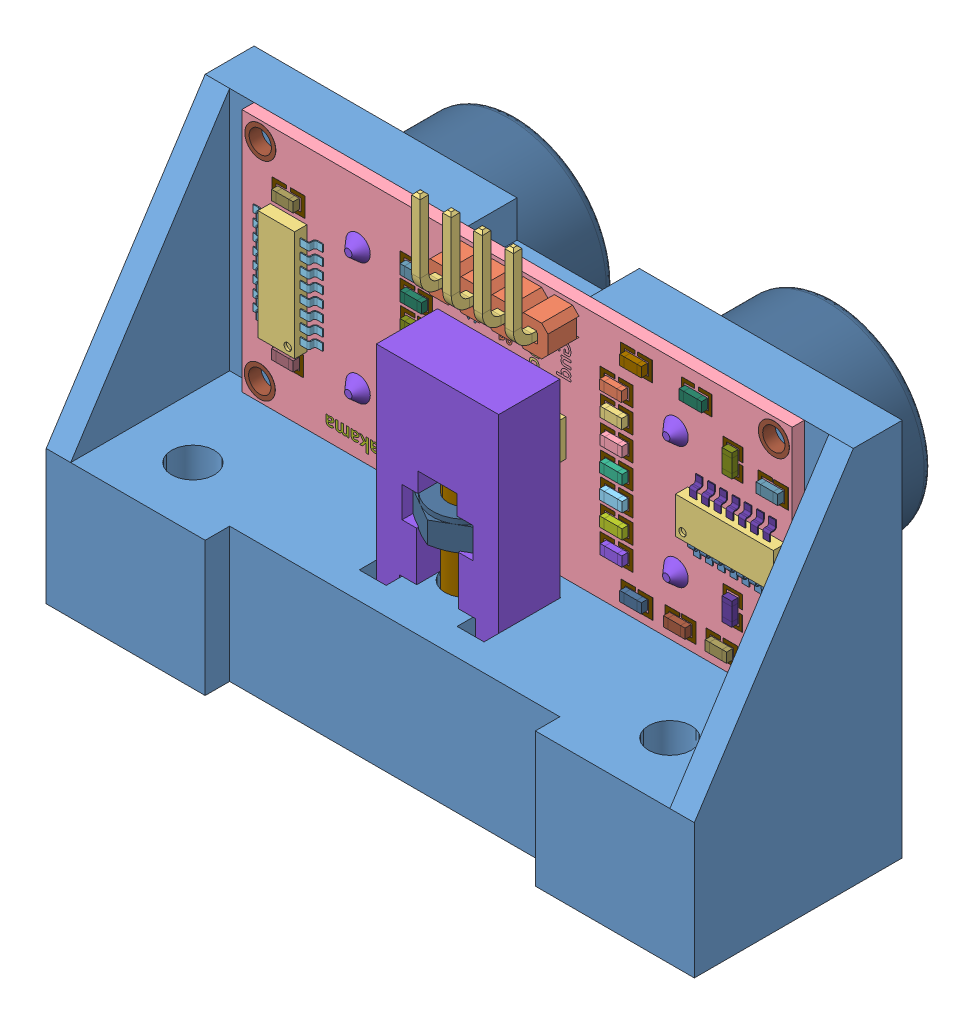
SolidWorks assembly cum_mat_hai_ben, configuration Default. Lengths in mm.
Overall size (53 36.57 25).
66 component instances, 64 part files, 9 mates.
Components (placement in the parent):
- ga lap ultrasonic v6-1: ga lap ultrasonic v6 [Default] at (-15.0838 26.1355 42.0068) size (53 31 17)
- HC-04HC-04-1: HC-04HC-04 [Default] at (-1.0033 34.8424 47.0068) x (1 0 0) z (0 0 -1) size (45 25.57 17.46)
  - HC-04HC-04.stp-1: HC-04HC-04.stp [Default] at origin size (45 25.57 17.46)
    - HC-04Array.stp-1: HC-04Array.stp [Default] at origin size (10.16 2.54 2.54)
    - HC-04Array001.stp-1: HC-04Array001.stp [Default] at (0 0 1) size (8.32 7.52 6.46)
    - HC-04Placa.stp-1: HC-04Placa.stp [Default] at origin size (45 20 1)
    - HC-04Pad003.stp-1: HC-04Pad003.stp [Default] at (0 0 1) size (10.52 3.38 0.2)
    - HC-04Fillet.stp-1: HC-04Fillet.stp [Default] at (0 0 1) size (10.1 2.84 3)
    - HC-04Array002.stp-1: HC-04Array002.stp [Default] at origin size (9.62 2 1)
    - HC-04Array003.stp-1: HC-04Array003.stp [Default] at (0 0 1) size (28 12 0.8)
    - HC-04Fusion.stp-1: HC-04Fusion.stp [Default] at origin size (6 2 1)
    - HC-04Fillet001.stp-1: HC-04Fillet001.stp [Default] at (0 0 1) size (42 16 12)
    - HC-04Pad005.stp-1: HC-04Pad005.stp [Default] at (0 0 1) size (39.16 13 0.2)
    - HC-04Pad006.stp-1: HC-04Pad006.stp [Default] at (0 0 1) size (35.01 9.04 7)
    - HC-04Fusion001.stp-1: HC-04Fusion001.stp [Default] at (0 0 8) size (31 5 1.5)
    - HC-04Clone_of_Fusion002.stp-1: HC-04Clone_of_Fusion002.stp [Default] at (47.2 -5.5 12.6) size (13 13 0.15)
    - HC-04Clone_of_Fusion003.stp-1: HC-04Clone_of_Fusion003.stp [Default] at (21.2 -5.5 12.6) size (13 13 0.15)
    - HC-04Array005.stp-1: HC-04Array005.stp [Default] at origin size (9.62 2 1)
    - HC-04Array002002.stp-1: HC-04Array002002.stp [Default] at (-5.9 0.1 0.15) size (6.57 1.4 0.56)
    - HC-04Clone_of_Array002002.stp-1: HC-04Clone_of_Array002002.stp [Default] at (-23.9 0.1 0.15) size (6.57 1.4 0.56)
    - HC-04Array002003.stp-1: HC-04Array002003.stp [Default] at (-6.05 0 0.15) size (6.57 1.4 0.56)
    - HC-04Clone_of_Array002003.stp-1: HC-04Clone_of_Array002003.stp [Default] at (-24.05 0 0.15) size (6.57 1.4 0.56)
    - HC-04Integrados.stp-1: HC-04Integrados.stp [Default] at origin size (42.14 9 1)
    - HC-04ShapeString.stp-1: HC-04ShapeString.stp [Default] at (-3.2 -7 1.01) x (0 1 0) z (0 0 1) size (2.53 1.13 0.01)
    - HC-04ShapeString001.stp-1: HC-04ShapeString001.stp [Default] at (-0.6 -7 1.01) x (0 1 0) z (0 0 1) size (2.66 1.45 0.01)
    - HC-04ShapeString002.stp-1: HC-04ShapeString002.stp [Default] at (1.9 -7 1.01) x (0 1 0) z (0 0 1) size (3.21 1.16 0.01)
    - HC-04ShapeString003.stp-1: HC-04ShapeString003.stp [Default] at (4.5 -7 1.01) x (0 1 0) z (0 0 1) size (2.71 1.16 0.01)
    - HC-04ShapeString004.stp-1: HC-04ShapeString004.stp [Default] at (-19.5 -9.3 1.01) size (1.84 2.34 0.01)
    - HC-04ShapeString005.stp-1: HC-04ShapeString005.stp [Default] at (17.5 -9.3 1.01) size (1.82 2.34 0.01)
    - HC-04ShapeString006.stp-1: HC-04ShapeString006.stp [Default] at (-3 3.7 1.01) size (5.52 1.41 0.01)
    - HC-04Pad008.stp-1: HC-04Pad008.stp [Default] at (0 0 -0.01) size (44.56 19.6 1.02)
    - HC-04Scale004.stp-1: HC-04Scale004.stp [Default] at (-1.9 -21.5 -1.5) x (0 1 0) z (0 0 1) size (0.8 1.77 0.5)
    - HC-04Scale027.stp-1: HC-04Scale027.stp [Default] at (-1.9 -10.2323 -1.5) x (0 1 0) z (0 0 1) size (0.8 1.77 0.5)
    - HC-04Scale028.stp-1: HC-04Scale028.stp [Default] at (8.5984 -21.5 -1.5) x (0 1 0) z (0 0 1) size (0.8 1.77 0.5)
    - HC-04Scale029.stp-1: HC-04Scale029.stp [Default] at (8.5984 -19.5867 -1.5) x (0 1 0) z (0 0 1) size (0.8 1.77 0.5)
    - HC-04Scale030.stp-1: HC-04Scale030.stp [Default] at (8.5984 -17.5982 -1.5) x (0 1 0) z (0 0 1) size (0.8 1.77 0.5)
    - HC-04Scale031.stp-1: HC-04Scale031.stp [Default] at (8.5984 -15.6427 -1.5) x (0 1 0) z (0 0 1) size (0.8 1.77 0.5)
    - HC-04Scale032.stp-1: HC-04Scale032.stp [Default] at (8.5984 -11.6848 -1.5) x (0 1 0) z (0 0 1) size (0.8 1.77 0.5)
    - HC-04Scale033.stp-1: HC-04Scale033.stp [Default] at (-26.74 -2 -1.5) x (0 1 0) z (0 0 1) size (0.8 1.85 0.5)
    - HC-04Scale034.stp-1: HC-04Scale034.stp [Default] at (24.9371 -21.5 -1.5) x (0 1 0) z (0 0 1) size (0.8 1.77 0.5)
    - HC-04Scale035.stp-1: HC-04Scale035.stp [Default] at (24.9691 -19.5867 -1.5) x (0 1 0) z (0 0 1) size (0.8 1.77 0.5)
    - HC-04Scale036.stp-1: HC-04Scale036.stp [Default] at (24.9742 -17.5982 -1.5) x (0 1 0) z (0 0 1) size (0.8 1.77 0.5)
    - HC-04Scale037.stp-1: HC-04Scale037.stp [Default] at (-10.4013 -2 -1.5) x (0 1 0) z (0 0 1) size (0.8 1.85 0.5)
    - HC-04Scale038.stp-1: HC-04Scale038.stp [Default] at (-10.4013 -3.9266 -1.5) x (0 1 0) z (0 0 1) size (0.8 1.85 0.5)
    - HC-04Scale039.stp-1: HC-04Scale039.stp [Default] at (-10.4013 -0.0734 -1.5) x (0 1 0) z (0 0 1) size (0.8 1.85 0.5)
    - HC-04Scale040.stp-1: HC-04Scale040.stp [Default] at (24.9742 -9.855 -1.5) x (0 1 0) z (0 0 1) size (0.8 1.77 0.5)
    - HC-04Scale041.stp-1: HC-04Scale041.stp [Default] at (26.5673 -24.0564 -1.5) x (0 1 0) z (0 0 1) size (0.8 1.77 0.5)
    - HC-04Scale042.stp-1: HC-04Scale042.stp [Default] at (26.5673 -7.3333 -1.5) x (0 1 0) z (0 0 1) size (0.8 1.77 0.5)
    - HC-04Scale043.stp-1: HC-04Scale043.stp [Default] at (30.1435 -7.3333 -1.5) x (0 1 0) z (0 0 1) size (0.8 1.77 0.5)
    - HC-04Scale044.stp-1: HC-04Scale044.stp [Default] at (33.5459 -7.3333 -1.5) x (0 1 0) z (0 0 1) size (0.8 1.77 0.5)
    - HC-04Scale045.stp-1: HC-04Scale045.stp [Default] at (37.7181 -11.1827 -1.5) x (0 1 0) z (0 0 1) size (0.8 1.77 0.5)
    - HC-04Scale046.stp-1: HC-04Scale046.stp [Default] at (37.7181 -20.5932 -1.5) x (0 1 0) z (0 0 1) size (0.8 1.77 0.5)
    - HC-04Scale047.stp-1: HC-04Scale047.stp [Default] at (-3.9042 -12.3288 -1.5) x (0 1 0) z (0 0 1) size (0.8 1.85 0.5)
    - HC-04Scale048.stp-1: HC-04Scale048.stp [Default] at (13.5402 13.2894 -1.5) size (0.8 1.85 0.5)
    - HC-04Scale049.stp-1: HC-04Scale049.stp [Default] at (13.5402 23.7909 -1.5) size (0.8 1.85 0.5)
    - HC-04Pad009.stp-1: HC-04Pad009.stp [Default] x (1 0 0) z (0 0 -1) size (42.21 18.43 0.01)
    - HC-04ShapeString007.stp-1: HC-04ShapeString007.stp [Default] at (-3.2 -7 -0.1) x (0 1 0) z (0 0 1) size (2.53 1.13 0.01)
    - HC-04ShapeString008.stp-1: HC-04ShapeString008.stp [Default] at (-0.6 -7 -0.1) x (0 1 0) z (0 0 1) size (2.66 1.45 0.01)
    - HC-04ShapeString009.stp-1: HC-04ShapeString009.stp [Default] at (1.9 -7 -0.1) x (0 1 0) z (0 0 1) size (3.21 1.16 0.01)
    - HC-04ShapeString010.stp-1: HC-04ShapeString010.stp [Default] at (4.5 -7 -0.1) x (0 1 0) z (0 0 1) size (2.71 1.16 0.01)
    - HC-04Fusion002.stp-1: HC-04Fusion002.stp [Default] at origin size (5.7 7.57 0.56)
    - HC-04ShapeString011.stp-1: HC-04ShapeString011.stp [Default] at (-17.5 8.4 1.1) size (7.91 1.16 0.01)
    - HC-04ShapeString012.stp-1: HC-04ShapeString012.stp [Default] at (-7.5 8 -0.1) x (-1 0 0) z (0 0 -1) size (7.91 1.16 0.01)
- 12.ganh-1: 12.ganh [Default] at (-1.0033 30.7424 48.5068) x (1 0 0) z (0 -1 0) size (10 5 19)
- countersunk flat head cross recess screw_iso-2: countersunk flat head cross recess screw_iso [ISO 7046-1 - M3 x 12 - Z - 12N] at (-1.0033 20.9424 51.1568) x (0 1 0) z (0 0 1) size (12 5.5 5.5)
- hex nut style 1 gradeab_iso-1: hex nut style 1 gradeab_iso [ISO - 4032 - M3 - W - N] at (-1.0033 28.6884 51.1568) x (1 0 0) z (0 -1 0) size (5.5 6.35 2.4)
Mates (geometry in assembly coordinates):
- Coincident1: coincident anti-aligned: plane of ga lap ultrasonic v6-1 through (-15.0838 26.1355 46.0068) normal (0 0 1); plane of HC-04HC-04-1/HC-04HC-04.stp-1/HC-04Placa.stp-1 through (-23.5033 24.8424 46.0068) normal (0 0 -1)
- Width1: width anti-aligned: plane of ga lap ultrasonic v6-1 through (-27.5033 44.8424 59.0068) normal (-1 0 0); plane of ga lap ultrasonic v6-1 through (25.4967 44.8424 59.0068) normal (1 0 0); plane of HC-04HC-04-1/HC-04HC-04.stp-1/HC-04Placa.stp-1 through (21.4967 24.8424 47.0068) normal (1 0 0); plane of HC-04HC-04-1/HC-04HC-04.stp-1/HC-04Placa.stp-1 through (-23.5033 44.8424 47.0068) normal (-1 0 0)
- Coincident2: coincident anti-aligned: plane of ga lap ultrasonic v6-1 through (-1.0033 24.8424 59.0068) normal (0 1 0); plane of HC-04HC-04-1/HC-04HC-04.stp-1/HC-04Placa.stp-1 through (-23.5033 24.8424 47.0068) normal (0 -1 0)
- Coincident3: coincident anti-aligned: plane of ga lap ultrasonic v6-1 through (4.0967 21.3424 48.5068) normal (0 0 1); plane of 12.ganh-1 through (-1.0033 30.7424 48.5068) normal (0 0 -1)
- Coincident4: coincident anti-aligned: plane of ga lap ultrasonic v6-1 through (-1.0033 24.8424 59.0068) normal (0 1 0); plane of 12.ganh-1 through (-1.0033 24.8424 53.5068) normal (0 -1 0)
- Width2: width aligned: plane of ga lap ultrasonic v6-1 through (4.0967 21.3424 48.5068) normal (-1 0 0); plane of ga lap ultrasonic v6-1 through (-6.1033 21.3424 48.5068) normal (1 0 0); plane of 12.ganh-1 through (-6.0033 30.7424 53.5068) normal (-1 0 0); plane of 12.ganh-1 through (3.9967 30.7424 53.5068) normal (1 0 0)
- Concentric1: concentric aligned: cylinder of ga lap ultrasonic v6-1 through (-1.0033 19.8424 51.1568) axis (0 1 0) radius 1.75; cone of countersunk flat head cross recess screw_iso-2 through (-1.0033 21.3424 51.1568) axis (0 1 0)
- Coincident6: coincident anti-aligned: plane of 12.ganh-1 through (-1.0033 32.9424 53.5068) normal (0 -1 0); plane of countersunk flat head cross recess screw_iso-2 through (-2.5033 32.9424 51.1568) normal (0 1 0)
- Concentric2: concentric aligned: cylinder of countersunk flat head cross recess screw_iso-2 through (-1.0033 14.5924 51.1568) axis (0 -1 0) radius 1.5; cylinder of hex nut style 1 gradeab_iso-1 through (-1.0033 53.7259 51.1568) axis (0 -1 0) radius 1.5
